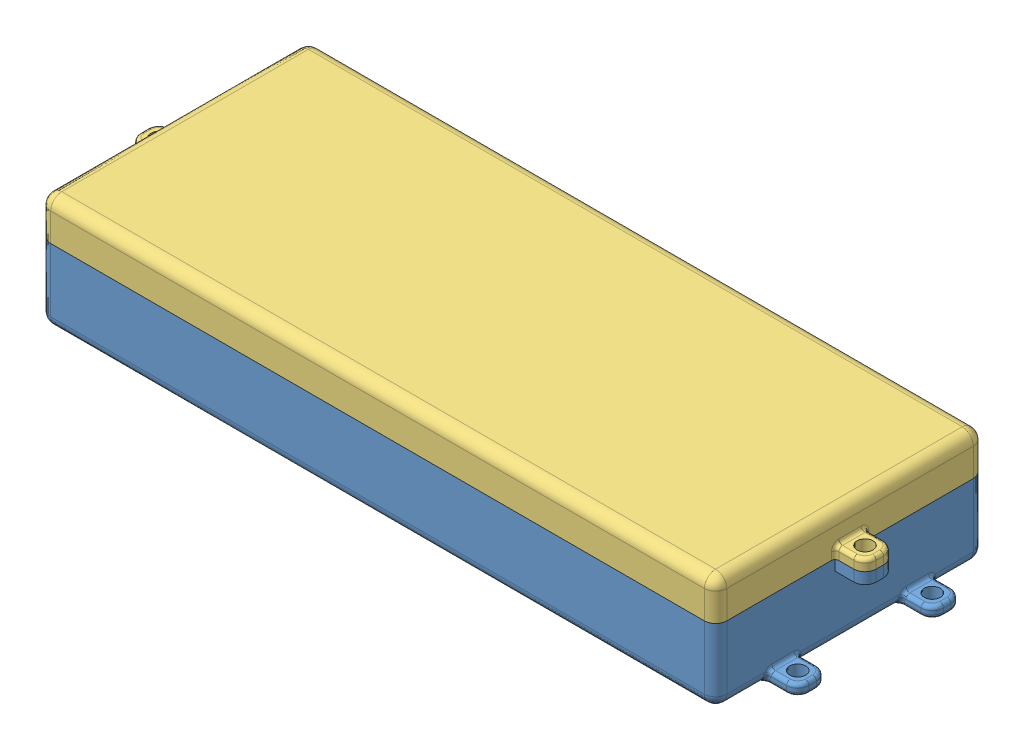
SolidWorks assembly Temp_Module, configuration Default. Lengths in mm.
Overall size (197 30.7 72).
3 component instances, 3 part files, 11 mates.
Components (placement in the parent):
- Temp_Module_Enclosure_Base-1: Temp_Module_Enclosure_Base [Default] at origin size (197 20.2 72)
- FSAES-22-E17 Temp Module PCB.step-1: FSAES-22-E17 Temp Module PCB.step [Default] at (-86.4111 14.3897 31.5516) x (1 0 0.000209) z (0 1 0) size (172.11 63.03 17.58)
- Temp_Module_Enclosure_Lid-1: Temp_Module_Enclosure_Lid [Default] at (0 20 0) size (197 10.5 72)
Mates (geometry in assembly coordinates):
- Coincident4: coordinate: point of Temp_Module_Enclosure_Base-1
- Parallel1: parallel anti-aligned: plane of Temp_Module_Enclosure_Base-1 through (0 3 0) normal (0 1 0); plane of FSAES-22-E17 Temp Module PCB.step-1 through (-0.4481 13 0.0471) normal (0 -1 0)
- Parallel2: parallel anti-aligned: plane of Temp_Module_Enclosure_Base-1 through (-87.5 20 -36) normal (1 0 0); plane of FSAES-22-E17 Temp Module PCB.step-1 through (-86.5 13 26.4716) normal (-1 0 0)
- Coincident12: coincident anti-aligned: plane of Temp_Module_Enclosure_Base-1 through (0 20 0) normal (0 1 0); plane of Temp_Module_Enclosure_Lid-1 through (0 20 0) normal (0 -1 0)
- Coincident13: coincident aligned: plane of Temp_Module_Enclosure_Base-1 through (-90.5 20 36) normal (0 0 1); plane of Temp_Module_Enclosure_Lid-1 through (-90.5 30.5 36) normal (0 0 1)
- Coincident14: coincident aligned: plane of Temp_Module_Enclosure_Base-1 through (-90.5 20 -36) normal (-1 0 0); plane of Temp_Module_Enclosure_Lid-1 through (-90.5 30.5 -36) normal (-1 0 0)
- Concentric1: concentric aligned: cylinder of Temp_Module_Enclosure_Base-1 through (-81.522 7 -26.4104) axis (0 1 0) radius 1.65; circle of FSAES-22-E17 Temp Module PCB.step-1
- Concentric2: concentric anti-aligned: cylinder of Temp_Module_Enclosure_Base-1 through (-81.432 7 26.4727) axis (0 1 0) radius 1.65; cylinder of FSAES-22-E17 Temp Module PCB.step-1 through (-81.432 13 26.4727) axis (0 -1 0) radius 1.65
- Concentric3: concentric aligned: cylinder of Temp_Module_Enclosure_Base-1 through (80.547 7 -26.3876) axis (0 1 0) radius 1.65; circle of FSAES-22-E17 Temp Module PCB.step-1
- Concentric4: concentric anti-aligned: cylinder of Temp_Module_Enclosure_Base-1 through (80.45 7 26.3644) axis (0 1 0) radius 1.65; cylinder of FSAES-22-E17 Temp Module PCB.step-1 through (80.45 13 26.3644) axis (0 -1 0) radius 1.65
- Coincident17: coincident anti-aligned: plane of Temp_Module_Enclosure_Base-1 through (0 13 0) normal (0 1 0); plane of FSAES-22-E17 Temp Module PCB.step-1 through (-0.4481 13 0.0471) normal (0 -1 0)
